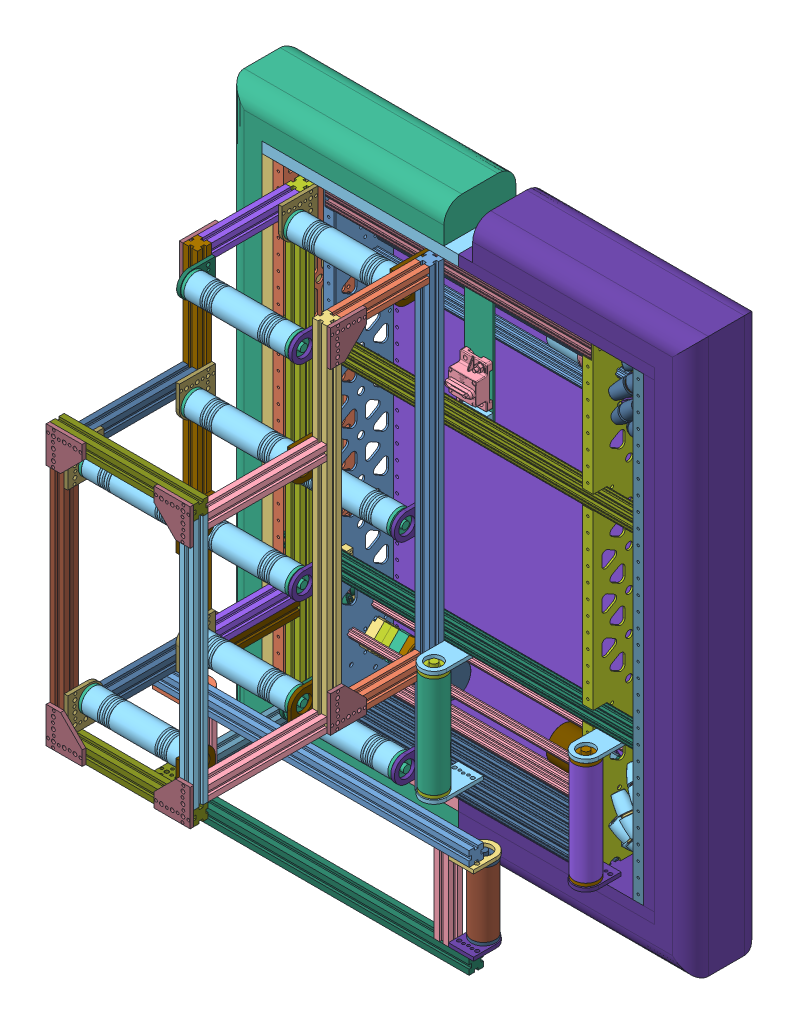
SolidWorks assembly Robot 2020, configuration Default. Lengths in mm. (continued)
Components (placement in the parent): (continued)
- Copy of Fame 2020-1: Copy of Fame 2020 [Default] at origin size (819.15 977.9 171.99) (continued)
  - Back Electronics Strap^Copy of Fame 2020-1: Back Electronics Strap^Copy of Fame 2020 [Default] at (0.05 266.7 84.65) x (0 1 0) z (0 0 1) size (228.6 81.6 66.64) (virtual) (continued)
    - am-0282 120a Circuit Breaker^Back Electronics Strap_Copy of Fame 2020-1: am-0282 120a Circuit Breaker^Back Electronics Strap_Copy of Fame 2020 [Default] at (-47.625 0 6.4135) x (1 0 0) z (0 -1 0) size (76.93 61.08 66.64) (virtual)
    - Electronics Strap Front Standoff^Back Electronics Strap_Copy of Fame 2020-1: Electronics Strap Front Standoff^Back Electronics Strap_Copy of Fame 2020 [Default] at (-101.6 0 7.1437) size (25.4 50.8 11.11) (virtual)
    - Back Electronics Strap-6^Back Electronics Strap_Copy of Fame 2020-1: Back Electronics Strap-6^Back Electronics Strap_Copy of Fame 2020 [Default] at origin size (228.6 50.8 3.17) (virtual)
  - Inner plate^Copy of Fame 2020-1: Inner plate^Copy of Fame 2020 [Default] at (212.725 0 58.7875) x (0 1 0) z (0 0 1) size (812.8 19.05 127) (virtual)
  - Base Plate^Copy of Fame 2020-1: Base Plate^Copy of Fame 2020 [Default] at origin size (469.9 812.8 3.17) (virtual)
  - 2.75_ Churro^Copy of Fame 2020-1: 2.75_ Churro^Copy of Fame 2020 [Default] at (238.125 -165.1 7.9875) x (0 0 -1) z (1 0 0) size (14.66 12.7 69.85) (virtual)
  - 1030-CL-16^Copy of Fame 2020-1: 1030-CL-16^Copy of Fame 2020 [Default] at (-184.1 -393.7 84.1875) x (0 -1 0) z (-1 0 0) size (25.4 76.2 469.9) (virtual)
  - 2.75_ Churro v1(Mirror) (2)^Copy of Fame 2020-1: 2.75_ Churro v1(Mirror) (2)^Copy of Fame 2020 [Default] at (238.125 165.1 7.9875) x (0 0 -1) z (-1 0 0) size (14.66 12.7 69.85) (virtual)
  - 2.75_ Churro v1(Mirror)^Copy of Fame 2020-1: 2.75_ Churro v1(Mirror)^Copy of Fame 2020 [Default] at (-238.125 -165.1 7.9875) x (0 0 -1) z (1 0 0) size (14.66 12.7 69.85) (virtual)
  - 1030-CL-16 v2(Mirror)^Copy of Fame 2020-1: 1030-CL-16 v2(Mirror)^Copy of Fame 2020 [Default] at (-184.1 393.7 84.1875) x (0 1 0) z (1 0 0) size (25.4 76.2 469.9) (virtual)
  - Outer plate^Copy of Fame 2020-1: Outer plate^Copy of Fame 2020 [Default] at (333.375 0 58.7875) x (0 -1 0) z (0 0 1) size (812.8 19.05 127) (virtual)
  - 1010-CL-22^Copy of Fame 2020-1: 1010-CL-22^Copy of Fame 2020 [Default] at (-257.175 -165.1 109.5875) x (0 0 1) z (-1 0 0) size (25.4 25.4 615.95) (virtual)
  - 1010-CL-22 v2(Mirror)^Copy of Fame 2020-1: 1010-CL-22 v2(Mirror)^Copy of Fame 2020 [Default] at (-257.175 165.1 109.5875) x (0 0 1) z (1 0 0) size (25.4 25.4 615.95) (virtual)
  - Bumper Assembly^Copy of Fame 2020-1: Bumper Assembly^Copy of Fame 2020 [Default] at (327.025 0.0665 58.7875) size (409.58 977.9 127) (virtual)
  - Inner Plate Cross Lock v4^Copy of Fame 2020-1: Inner Plate Cross Lock v4^Copy of Fame 2020 [Default] at (235 -165.1 96.8875) x (0 1 0) z (0 0 1) size (25.4 12.7 12.7) (virtual)
  - Motor Brace^Copy of Fame 2020-1: Motor Brace^Copy of Fame 2020 [Default] at (120.6 292.8812 76.0284) x (0 0 1) z (-1 0 0) size (14.66 12.7 470) (virtual)
  - Inner Plate Cross Lock v4 v1(Mirror) (2)^Copy of Fame 2020-1: Inner Plate Cross Lock v4 v1(Mirror) (2)^Copy of Fame 2020 [Default] at (235 165.1 96.8875) x (0 -1 0) z (0 0 -1) size (25.4 12.7 12.7) (virtual)
  - Inner Plate Cross Lock v4 v1(Mirror)^Copy of Fame 2020-1: Inner Plate Cross Lock v4 v1(Mirror)^Copy of Fame 2020 [Default] at (-235 -165.1 96.8875) x (0 1 0) z (0 0 -1) size (25.4 12.7 12.7) (virtual)
  - Motor Brace^Copy of Fame 2020-2: Motor Brace^Copy of Fame 2020 [Default] at (-69.8 342.1188 76.0284) x (0 0 -1) z (1 0 0) size (14.66 12.7 470) (virtual)
  - Motor Brace^Copy of Fame 2020-3: Motor Brace^Copy of Fame 2020 [Default] at (120.6 268.2625 33.3875) x (0 0 1) z (-1 0 0) size (14.66 12.7 470) (virtual)
  - Motor Brace^Copy of Fame 2020-4: Motor Brace^Copy of Fame 2020 [Default] at (-69.8 366.7375 33.3875) x (0 0 -1) z (1 0 0) size (14.66 12.7 470) (virtual)
  - Motor Brace v1(Mirror)^Copy of Fame 2020-1: Motor Brace v1(Mirror)^Copy of Fame 2020 [Default] at (120.6 -292.8812 76.0284) x (0 0 1) z (1 0 0) size (14.66 12.7 470) (virtual)
  - Motor Brace v1(Mirror)^Copy of Fame 2020-2: Motor Brace v1(Mirror)^Copy of Fame 2020 [Default] at (-69.8 -342.1188 76.0284) x (0 0 -1) z (-1 0 0) size (14.66 12.7 470) (virtual)
  - Motor Brace v1(Mirror)^Copy of Fame 2020-3: Motor Brace v1(Mirror)^Copy of Fame 2020 [Default] at (120.6 -268.2625 33.3875) x (0 0 1) z (1 0 0) size (14.66 12.7 470) (virtual)
  - Motor Brace v1(Mirror)^Copy of Fame 2020-4: Motor Brace v1(Mirror)^Copy of Fame 2020 [Default] at (-69.8 -366.7375 33.3875) x (0 0 -1) z (-1 0 0) size (14.66 12.7 470) (virtual)
- Copy of Snake-1: Copy of Snake [Default] at (-279.4 -406.4 122.2875) x (0 -1 0) z (0 0 1) size (812.8 266.7 447.68)
  - RollerALL-1: RollerALL [Default] at (-406.4 279.4 -122.2875) size (42.07 203.2 42.07)
    - Roller-1: Roller [Default] at (366.7125 -241.3 161.975) size (42.07 177.8 42.07)
    - RollerEndCap-3: RollerEndCap [Default] at (366.7125 -247.65 161.975) size (42.07 25.4 42.07)
    - RollerEndCap-2: RollerEndCap [Default] at (366.7125 -57.15 161.975) x (1 0 0) z (0 0 -1) size (42.07 25.4 42.07)
  - RollerALL-3: RollerALL [Default] at (-958.85 278.4 58.6875) size (42.07 203.2 42.07)
    - Roller-1: Roller [Default] at (366.7125 -241.3 161.975) size (42.07 177.8 42.07)
    - RollerEndCap-3: RollerEndCap [Default] at (366.7125 -247.65 161.975) size (42.07 25.4 42.07)
    - RollerEndCap-2: RollerEndCap [Default] at (366.7125 -57.15 161.975) x (1 0 0) z (0 0 -1) size (42.07 25.4 42.07)
  - RollerALL-4: RollerALL [Default] at (-777.875 278.4 58.6875) size (42.07 203.2 42.07)
    - Roller-1: Roller [Default] at (366.7125 -241.3 161.975) size (42.07 177.8 42.07)
    - RollerEndCap-3: RollerEndCap [Default] at (366.7125 -247.65 161.975) size (42.07 25.4 42.07)
    - RollerEndCap-2: RollerEndCap [Default] at (366.7125 -57.15 161.975) x (1 0 0) z (0 0 -1) size (42.07 25.4 42.07)
  - RollerALL-5: RollerALL [Default] at (-958.85 278.4 239.6625) size (42.07 203.2 42.07)
    - Roller-1: Roller [Default] at (366.7125 -241.3 161.975) size (42.07 177.8 42.07)
    - RollerEndCap-3: RollerEndCap [Default] at (366.7125 -247.65 161.975) size (42.07 25.4 42.07)
    - RollerEndCap-2: RollerEndCap [Default] at (366.7125 -57.15 161.975) x (1 0 0) z (0 0 -1) size (42.07 25.4 42.07)
  - RollerALL-6: RollerALL [Default] at (-1139.825 278.4 -122.2875) size (42.07 203.2 42.07)
    - Roller-1: Roller [Default] at (366.7125 -241.3 161.975) size (42.07 177.8 42.07)
    - RollerEndCap-3: RollerEndCap [Default] at (366.7125 -247.65 161.975) size (42.07 25.4 42.07)
    - RollerEndCap-2: RollerEndCap [Default] at (366.7125 -57.15 161.975) x (1 0 0) z (0 0 -1) size (42.07 25.4 42.07)
  - RollerALL-7: RollerALL [Default] at (-1139.825 278.4 58.6875) size (42.07 203.2 42.07)
    - Roller-1: Roller [Default] at (366.7125 -241.3 161.975) size (42.07 177.8 42.07)
    - RollerEndCap-3: RollerEndCap [Default] at (366.7125 -247.65 161.975) size (42.07 25.4 42.07)
    - RollerEndCap-2: RollerEndCap [Default] at (366.7125 -57.15 161.975) x (1 0 0) z (0 0 -1) size (42.07 25.4 42.07)
  - RollerALL-8: RollerALL [Default] at (-777.875 277.3088 -122.2875) size (42.07 203.2 42.07)
    - Roller-1: Roller [Default] at (366.7125 -241.3 161.975) size (42.07 177.8 42.07)
    - RollerEndCap-3: RollerEndCap [Default] at (366.7125 -247.65 161.975) size (42.07 25.4 42.07)
    - RollerEndCap-2: RollerEndCap [Default] at (366.7125 -57.15 161.975) x (1 0 0) z (0 0 -1) size (42.07 25.4 42.07)
  - RollerALL-9: RollerALL [Default] at (-596.9 278.4 58.6875) size (42.07 203.2 42.07)
    - Roller-1: Roller [Default] at (366.7125 -241.3 161.975) size (42.07 177.8 42.07)
    - RollerEndCap-3: RollerEndCap [Default] at (366.7125 -247.65 161.975) size (42.07 25.4 42.07)
    - RollerEndCap-2: RollerEndCap [Default] at (366.7125 -57.15 161.975) x (1 0 0) z (0 0 -1) size (42.07 25.4 42.07)
  - RollerALL-10: RollerALL [Default] at (-596.9 278.4 239.6625) size (42.07 203.2 42.07)
    - Roller-1: Roller [Default] at (366.7125 -241.3 161.975) size (42.07 177.8 42.07)
    - RollerEndCap-3: RollerEndCap [Default] at (366.7125 -247.65 161.975) size (42.07 25.4 42.07)
    - RollerEndCap-2: RollerEndCap [Default] at (366.7125 -57.15 161.975) x (1 0 0) z (0 0 -1) size (42.07 25.4 42.07)
  - 1010-32^Copy of Snake-1: 1010-32^Copy of Snake [Default] at (0 12.7 12.7) x (0 0 1) z (-1 0 0) size (25.4 25.4 812.8) (virtual)
  - 1010-6.125^Copy of Snake-1: 1010-6.125^Copy of Snake [Default] at (-800.1 12.7 25.4) size (25.4 25.4 155.57) (virtual)
  - 1010-6.125^Copy of Snake-2: 1010-6.125^Copy of Snake [Default] at (-203.2 12.7 25.4) size (25.4 25.4 155.57) (virtual)
  - 1010-24.5^Copy of Snake-1: 1010-24.5^Copy of Snake [Default] at (-190.5 12.7 193.675) x (0 0 1) z (-1 0 0) size (25.4 25.4 622.3) (virtual)
  - 1010-8.25^Copy of Snake-1: 1010-8.25^Copy of Snake [Default] at (-203.2 12.7 206.375) size (25.4 25.4 209.55) (virtual)
  - 1010-8.25^Copy of Snake-2: 1010-8.25^Copy of Snake [Default] at (-619.125 12.7 206.375) size (25.4 25.4 209.55) (virtual)
  - 1010-17.375^Copy of Snake-1: 1010-17.375^Copy of Snake [Default] at (-190.5 12.7 428.625) x (0 0 1) z (-1 0 0) size (25.4 25.4 441.33) (virtual)
  - Corner Bearing Bracket^Copy of Snake-1: Corner Bearing Bracket^Copy of Snake [Default] at (-812.8 25.4 0) size (63.5 6.35 63.5) (virtual)
  - Corner Bearing Bracket^Copy of Snake-2: Corner Bearing Bracket^Copy of Snake [Default] at (-631.825 25.4 441.325) x (0 0 -1) z (1 0 0) size (63.5 6.35 63.5) (virtual)
  - Corner Bearing Bracket^Copy of Snake-3: Corner Bearing Bracket^Copy of Snake [Default] at (-190.5 25.4 441.325) x (-1 0 0) z (0 0 -1) size (63.5 6.35 63.5) (virtual)
  - Corner Bearing Bracket^Copy of Snake-4: Corner Bearing Bracket^Copy of Snake [Default] at (-190.5 25.4 180.975) x (0 0 1) z (-1 0 0) size (63.5 6.35 63.5) (virtual)
  - Corner Bearing Bracket^Copy of Snake-5: Corner Bearing Bracket^Copy of Snake [Default] at (-631.825 25.4 180.975) size (63.5 6.35 63.5) (virtual)
  - CornerBracket-5: CornerBracket [Default] at (-190.5 0 206.375) x (-1 0 0) z (0 0 1) size (63.5 6.35 63.5)
  - CornerBracket-6: CornerBracket [Default] at (-812.8 0 206.375) x (0 0 -1) z (-1 0 0) size (63.5 6.35 63.5)
  - CornerBracket-7: CornerBracket [Default] at (-657.225 0 447.675) x (0 1 0) z (-1 0 0) size (63.5 6.35 63.5)
  - CornerBracket-8: CornerBracket [Default] at (-165.1 0 447.675) x (-1 0 0) z (0 -1 0) size (63.5 6.35 63.5)
  - CenterRollerBracket-1: CenterRollerBracket [Default] at (-388.9375 24.3088 0) x (-1 0 0) z (0 0 -1) size (44.45 6.35 61.91)
  - Center Bearing Bracket^Copy of Snake-2: Center Bearing Bracket^Copy of Snake [Default] at (-433.3875 25.4 180.975) size (44.45 6.35 61.91) (virtual)
  - Center Bearing Bracket^Copy of Snake-3: Center Bearing Bracket^Copy of Snake [Default] at (-795.3375 25.4 180.975) size (44.45 6.35 61.91) (virtual)
  - Center Bearing Bracket^Copy of Snake-4: Center Bearing Bracket^Copy of Snake [Default] at (-61.9125 25.4 0) size (44.45 6.35 61.91) (virtual)
  - 1010-10^Copy of Snake-1: 1010-10^Copy of Snake [Default] at (-177.8 0 428.625) x (1 0 0) z (0 1 0) size (25.4 25.4 254) (virtual)
  - 1010-10^Copy of Snake-2: 1010-10^Copy of Snake [Default] at (-644.525 0 428.625) x (1 0 0) z (0 1 0) size (25.4 25.4 254) (virtual)
  - Center Bearing Bracket v1(Mirror)^Copy of Snake-1: Center Bearing Bracket v1(Mirror)^Copy of Snake [Default] at (-433.3875 228.6 0) x (1 0 0) z (0 0 -1) size (44.45 6.35 61.91) (virtual)
  - Center Bearing Bracket v1(Mirror)^Copy of Snake-2: Center Bearing Bracket v1(Mirror)^Copy of Snake [Default] at (-433.3875 228.6 180.975) x (1 0 0) z (0 0 -1) size (44.45 6.35 61.91) (virtual)
  - Center Bearing Bracket v1(Mirror)^Copy of Snake-3: Center Bearing Bracket v1(Mirror)^Copy of Snake [Default] at (-795.3375 228.6 180.975) x (1 0 0) z (0 0 -1) size (44.45 6.35 61.91) (virtual)
  - Center Bearing Bracket v1(Mirror)^Copy of Snake-4: Center Bearing Bracket v1(Mirror)^Copy of Snake [Default] at (-61.9125 228.6 0) x (1 0 0) z (0 0 -1) size (44.45 6.35 61.91) (virtual)
  - Corner Bearing Bracket v1(Mirror) (1)^Copy of Snake-1: Corner Bearing Bracket v1(Mirror) (1)^Copy of Snake [Default] at (-812.8 228.6 0) x (1 0 0) z (0 0 -1) size (63.5 6.35 63.5) (virtual)
  - Corner Bearing Bracket v1(Mirror) (1)^Copy of Snake-2: Corner Bearing Bracket v1(Mirror) (1)^Copy of Snake [Default] at (-631.825 228.6 441.325) x (0 0 -1) z (-1 0 0) size (63.5 6.35 63.5) (virtual)
  - Corner Bearing Bracket v1(Mirror) (1)^Copy of Snake-3: Corner Bearing Bracket v1(Mirror) (1)^Copy of Snake [Default] at (-190.5 228.6 441.325) x (-1 0 0) z (0 0 1) size (63.5 6.35 63.5) (virtual)
  - Corner Bearing Bracket v1(Mirror) (1)^Copy of Snake-4: Corner Bearing Bracket v1(Mirror) (1)^Copy of Snake [Default] at (-190.5 228.6 180.975) x (0 0 1) z (1 0 0) size (63.5 6.35 63.5) (virtual)
  - Corner Bearing Bracket v1(Mirror) (1)^Copy of Snake-5: Corner Bearing Bracket v1(Mirror) (1)^Copy of Snake [Default] at (-631.825 228.6 180.975) x (1 0 0) z (0 0 -1) size (63.5 6.35 63.5) (virtual)
  - 1010-32 v1(Mirror)^Copy of Snake-1: 1010-32 v1(Mirror)^Copy of Snake [Default] at (0 241.3 12.7) x (0 0 1) z (1 0 0) size (25.4 25.4 812.8) (virtual)
  - 1010-6.125 v1(Mirror)^Copy of Snake-1: 1010-6.125 v1(Mirror)^Copy of Snake [Default] at (-800.1 241.3 25.4) x (1 0 0) z (0 0 -1) size (25.4 25.4 155.57) (virtual)
  - 1010-6.125 v1(Mirror)^Copy of Snake-2: 1010-6.125 v1(Mirror)^Copy of Snake [Default] at (-203.2 241.3 25.4) x (1 0 0) z (0 0 -1) size (25.4 25.4 155.57) (virtual)
  - 1010-24.5 v1(Mirror)^Copy of Snake-1: 1010-24.5 v1(Mirror)^Copy of Snake [Default] at (-190.5 241.3 193.675) x (0 0 1) z (1 0 0) size (25.4 25.4 622.3) (virtual)
  - 1010-8.25 v1(Mirror)^Copy of Snake-1: 1010-8.25 v1(Mirror)^Copy of Snake [Default] at (-203.2 241.3 206.375) x (1 0 0) z (0 0 -1) size (25.4 25.4 209.55) (virtual)
  - 1010-8.25 v1(Mirror)^Copy of Snake-2: 1010-8.25 v1(Mirror)^Copy of Snake [Default] at (-619.125 241.3 206.375) x (1 0 0) z (0 0 -1) size (25.4 25.4 209.55) (virtual)
  - 1010-17.375 v1(Mirror)^Copy of Snake-1: 1010-17.375 v1(Mirror)^Copy of Snake [Default] at (-190.5 241.3 428.625) x (0 0 1) z (1 0 0) size (25.4 25.4 441.33) (virtual)
  - CornerBracket-1: CornerBracket [Default] at (-190.5 260.35 206.375) x (-1 0 0) z (0 0 1) size (63.5 6.35 63.5)
  - CornerBracket-2: CornerBracket [Default] at (-812.8 260.35 206.375) x (0 0 -1) z (-1 0 0) size (63.5 6.35 63.5)
  - CornerBracket-3: CornerBracket [Default] at (-657.225 254 447.675) x (1 0 0) z (0 1 0) size (63.5 6.35 63.5)
  - CornerBracket-4: CornerBracket [Default] at (-165.1 254 447.675) x (0 -1 0) z (1 0 0) size (63.5 6.35 63.5)
- Copy of Serializer-1: Copy of Serializer [Default] at (-279.4 -406.4 96.8875) size (566.74 228.6 285.75)
  - Roller_9^Copy of Serializer_Robot 2020-1: Roller_9^Copy of Serializer_Robot 2020 [Default] at origin size (42.07 203.2 42.07) (virtual)
    - Roller 7^Roller_9_Copy of Serializer_Robot 2020-1: Roller 7^Roller_9_Copy of Serializer_Robot 2020 [Default] at (276.225 38.1 65.0875) size (42.07 177.8 42.07) (virtual)
    - Roller Hub^Roller_9_Copy of Serializer_Robot 2020-1: Roller Hub^Roller_9_Copy of Serializer_Robot 2020 [Default] at (276.225 31.75 65.0875) size (42.07 25.4 42.07) (virtual)
    - Roller Hub^Roller_9_Copy of Serializer_Robot 2020-2: Roller Hub^Roller_9_Copy of Serializer_Robot 2020 [Default] at (276.225 222.25 65.0875) x (1 0 0) z (0 0 -1) size (42.07 25.4 42.07) (virtual)
  - Roller_10^Copy of Serializer_Robot 2020-1: Roller_10^Copy of Serializer_Robot 2020 [Default] at origin size (42.07 203.2 42.07) (virtual)
    - Roller 7^Roller_10_Copy of Serializer_Robot 2020-1: Roller 7^Roller_10_Copy of Serializer_Robot 2020 [Default] at (544.5125 38.1 65.0875) size (42.07 177.8 42.07) (virtual)
    - Roller Hub^Roller_10_Copy of Serializer_Robot 2020-1: Roller Hub^Roller_10_Copy of Serializer_Robot 2020 [Default] at (544.5125 31.75 65.0875) size (42.07 25.4 42.07) (virtual)
    - Roller Hub^Roller_10_Copy of Serializer_Robot 2020-2: Roller Hub^Roller_10_Copy of Serializer_Robot 2020 [Default] at (544.5125 222.25 65.0875) x (1 0 0) z (0 0 -1) size (42.07 25.4 42.07) (virtual)
  - Roller Short^Copy of Serializer_Robot 2020-1: Roller Short^Copy of Serializer_Robot 2020 [Default] at origin size (42.07 139.7 42.07) (virtual)
    - Roller Hub^Roller Short_Copy of Serializer_Robot 2020-1: Roller Hub^Roller Short_Copy of Serializer_Robot 2020 [Default] at (544.5125 31.75 246.0625) size (42.07 25.4 42.07) (virtual)
    - Roller 4.5^Roller Short_Copy of Serializer_Robot 2020-1: Roller 4.5^Roller Short_Copy of Serializer_Robot 2020 [Default] at (544.5125 38.1 246.0625) size (42.07 114.3 42.07) (virtual)
    - Roller Hub^Roller Short_Copy of Serializer_Robot 2020-2: Roller Hub^Roller Short_Copy of Serializer_Robot 2020 [Default] at (544.5125 158.75 246.0625) x (1 0 0) z (0 0 -1) size (42.07 25.4 42.07) (virtual)
  - Roller Short_1^Copy of Serializer_Robot 2020-1: Roller Short_1^Copy of Serializer_Robot 2020 [Default] at origin size (42.07 139.7 42.07) (virtual)
    - Roller Hub^Roller Short_1_Copy of Serializer_Robot 2020-1: Roller Hub^Roller Short_1_Copy of Serializer_Robot 2020 [Default] at (39.6875 31.75 246.0625) size (42.07 25.4 42.07) (virtual)
    - Roller 4.5^Roller Short_1_Copy of Serializer_Robot 2020-1: Roller 4.5^Roller Short_1_Copy of Serializer_Robot 2020 [Default] at (39.6875 38.1 246.0625) size (42.07 114.3 42.07) (virtual)
    - Roller Hub^Roller Short_1_Copy of Serializer_Robot 2020-2: Roller Hub^Roller Short_1_Copy of Serializer_Robot 2020 [Default] at (39.6875 158.75 246.0625) x (1 0 0) z (0 0 -1) size (42.07 25.4 42.07) (virtual)
  - 1010-8.25^Copy of Serializer_Robot 2020-1: 1010-8.25^Copy of Serializer_Robot 2020 [Default] at (12.7 12.7 50.8) size (25.4 25.4 209.55) (virtual)
  - 1010-22^Copy of Serializer_Robot 2020-1: 1010-22^Copy of Serializer_Robot 2020 [Default] at (0 12.7 273.05) x (0 0 -1) z (1 0 0) size (25.4 25.4 558.8) (virtual)
  - Corner Bearing Bracket^Copy of Serializer_Robot 2020-1: Corner Bearing Bracket^Copy of Serializer_Robot 2020 [Default] at (0 25.4 285.75) x (0 0 -1) z (1 0 0) size (63.5 6.35 63.5) (virtual)
  - Center Bearing Bracket^Copy of Serializer_Robot 2020-1: Center Bearing Bracket^Copy of Serializer_Robot 2020 [Default] at (522.2875 25.4 25.4) size (44.45 6.35 61.91) (virtual)
  - Center Bearing Bracket^Copy of Serializer_Robot 2020-2: Center Bearing Bracket^Copy of Serializer_Robot 2020 [Default] at (566.7375 25.4 285.75) x (-1 0 0) z (0 0 -1) size (44.45 6.35 61.91) (virtual)
  - 1010-8.25 v1(Mirror)_1^Copy of Serializer_Robot 2020-1: 1010-8.25 v1(Mirror)_1^Copy of Serializer_Robot 2020 [Default] at (12.7 177.8 50.8) x (1 0 0) z (0 0 -1) size (25.4 25.4 209.55) (virtual)
  - 1010-22 v1(Mirror)^Copy of Serializer_Robot 2020-1: 1010-22 v1(Mirror)^Copy of Serializer_Robot 2020 [Default] at (0 177.8 273.05) x (0 0 -1) z (-1 0 0) size (25.4 25.4 558.8) (virtual)
  - Corner Bearing Bracket v2(Mirror)^Copy of Serializer_Robot 2020-1: Corner Bearing Bracket v2(Mirror)^Copy of Serializer_Robot 2020 [Default] at (0 165.1 285.75) x (0 0 -1) z (-1 0 0) size (63.5 6.35 63.5) (virtual)
  - Center Bearing Bracket v3(Mirror)^Copy of Serializer_Robot 2020-1: Center Bearing Bracket v3(Mirror)^Copy of Serializer_Robot 2020 [Default] at (566.7375 165.1 285.75) x (-1 0 0) z (0 0 1) size (44.45 6.35 61.91) (virtual)
  - 1010-5.5^Copy of Serializer_Robot 2020-1: 1010-5.5^Copy of Serializer_Robot 2020 [Default] at (76.2 25.4 273.05) x (1 0 0) z (0 1 0) size (25.4 25.4 139.7) (virtual)
  - 1010-5.5^Copy of Serializer_Robot 2020-2: 1010-5.5^Copy of Serializer_Robot 2020 [Default] at (509.5875 165.1 273.05) x (1 0 0) z (0 -1 0) size (25.4 25.4 139.7) (virtual)
  - Center Bearing Bracket Tall^Copy of Serializer_Robot 2020-1: Center Bearing Bracket Tall^Copy of Serializer_Robot 2020 [Default] at (254 222.25 0) size (44.45 6.35 87.31) (virtual)
  - Center Bearing Bracket Tall^Copy of Serializer_Robot 2020-2: Center Bearing Bracket Tall^Copy of Serializer_Robot 2020 [Default] at (522.2875 222.25 0) size (44.45 6.35 87.31) (virtual)
  - Center Bearing Bracket Tall^Copy of Serializer_Robot 2020-3: Center Bearing Bracket Tall^Copy of Serializer_Robot 2020 [Default] at (254 25.4 0) size (44.45 6.35 87.31) (virtual)
